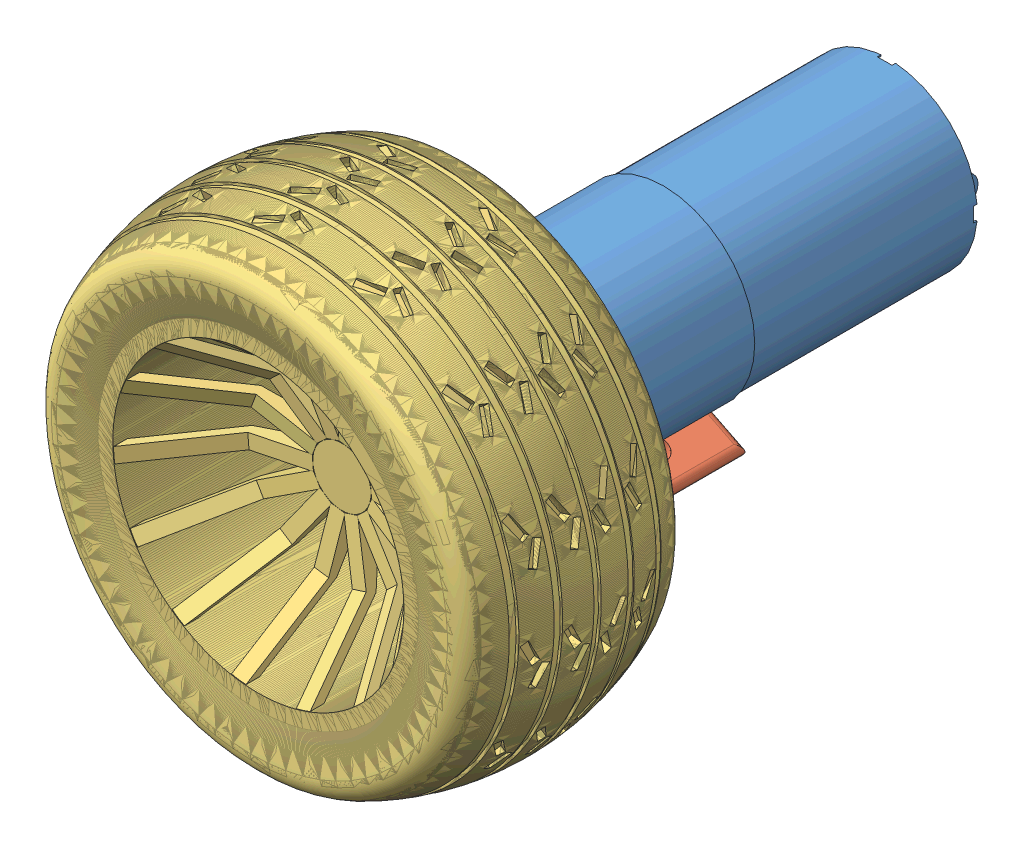
SolidWorks assembly Motor assembly, configuration Default. Lengths in mm.
Overall size (81.67 81.67 90.74).
5 component instances, 4 part files, 12 mates.
Components (placement in the parent):
- dc motor-1: dc motor [Default] at (29.3048 35.2797 20.0121) size (25 25 72.3)
- new motor holder-1: new motor holder [Default] at (32.8529 14.4792 73.8121) x (-0.89379 0.448485 0) z (0 0 -1) size (25 31.5 33)
- tire-2: tire [Défaut] at (29.3048 35.2797 92.3578) x (0 0 -1) z (-0.952681 -0.303972 0) size (29.78 64.99 64.99)
- bolt-1: bolt [Default] at (36.902 31.4676 76.4477) x (-0.31031 -0.950635 0) z (0 0 -1) size (5.19 4.62 12)
- bolt-2: bolt [Default] at (21.7075 39.0918 76.1821) x (0.923728 0.383049 0) z (0 0 -1) size (5.19 4.62 12)
Mates (geometry in assembly coordinates):
- Coincident1: coincident anti-aligned: circle of dc motor-1; circle of new motor holder-1
- Concentric3: concentric aligned: circle of new motor holder-1; circle of bolt-2
- Concentric5: concentric aligned: circle of new motor holder-1; circle of bolt-1
- Coincident5: coincident anti-aligned: circle of dc motor-1; circle of tire-2
- Coincident14: coincident anti-aligned: circle of dc motor-1; circle of new motor holder-1
- Concentric14: concentric aligned: circle of new motor holder-1; circle of bolt-2
- Concentric15: concentric aligned: circle of new motor holder-1; circle of bolt-1
- Coincident15: coincident anti-aligned: circle of dc motor-1; circle of tire-2
- Coincident16: coincident anti-aligned: circle of dc motor-1; circle of new motor holder-1
- Concentric16: concentric aligned: circle of new motor holder-1; circle of bolt-2
- Concentric17: concentric aligned: circle of new motor holder-1; circle of bolt-1
- Coincident17: coincident anti-aligned: circle of dc motor-1; circle of tire-2
